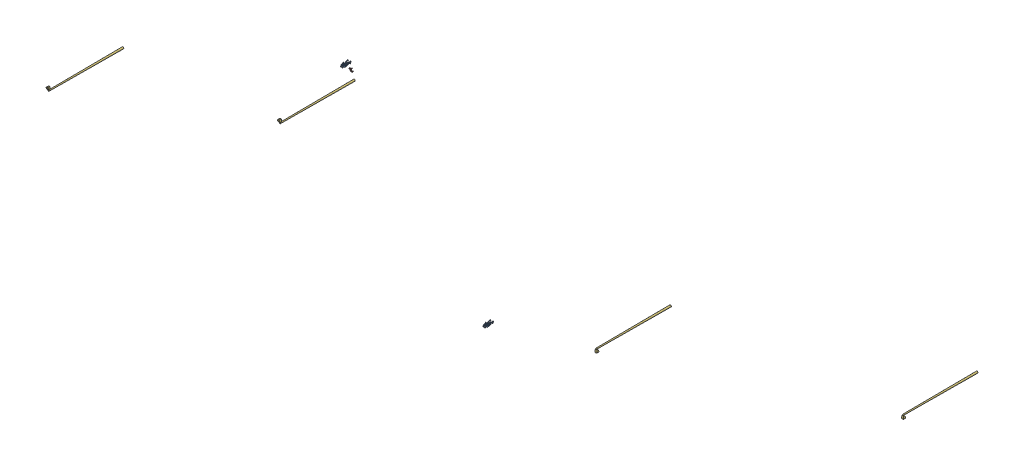
SolidWorks assembly Park scene, configuration Default. Lengths in mm.
Overall size (172997.33 40708.96 15155.93).
7 component instances, 3 part files, 8 mates.
Components (placement in the parent):
- Couple Walking v2-1: Couple Walking v2 [Default] at (97042.8871 20768.0893 0) size (971.22 682.9 1718.91)
- Couple Walking v2-2: Couple Walking v2 [Default] at (68307.1667 51803.1052 0) size (971.22 682.9 1718.91)
- German Shepherd-1: German Shepherd [Predeterminado] at (69037.0009 50613.5051 -995.4825) x (-0.927424 -0.373877 -0.010044) z (-0.373704 0.927415 -0.015684) size (212.95 642.55 996.13)
- LightPole-1: LightPole [Default] at (22635.286 31390.4456 0) x (-0.361809 0.932252 0) z (0 0 1) size (771.46 400 15150.67)
- LightPole-2: LightPole [Default] at (69285.9057 49048.0785 0) x (-0.361809 0.932252 0) z (0 0 1) size (771.46 400 15150.67)
- LightPole-3: LightPole [Default] at (133048.7527 41507.2409 0) x (0.217287 -0.976108 0) z (0 0 1) size (771.46 400 15150.67)
- LightPole-4: LightPole [Default] at (194905.5352 60880.401 0) x (0.217287 -0.976108 0) z (0 0 1) size (771.46 400 15150.67)
Mates (geometry in assembly coordinates):
- Coincident1: coincident anti-aligned: plane of Viaduct-1 through (121720.7023 -158145.4536 0) normal (0 0 -1)
- Coincident3: coincident: point of Viaduct-1
- Parallel1: parallel anti-aligned: plane of Viaduct-1 through (127159.1693 53321.2792 3923.6765) normal (0 -1 0)
- Coincident5: coincident aligned: plane of Couple Walking v2-1 through (97042.8871 20768.0893 0) normal (0 0 1)
- Coincident6: coincident aligned: plane of Couple Walking v2-2 through (68307.1667 51803.1052 0) normal (0 0 1)
- Tangent3: tangent anti-aligned: plane of Couple Walking v2-2 through (68307.1667 51803.1052 0) normal (0 0 1); face of German Shepherd-1
- Coincident7: coincident aligned: plane of LightPole-1 through (22635.286 31390.4456 0) normal (0 0 1)
- Coincident14: coincident aligned: plane of LightPole-3 through (133048.7527 41507.2409 0) normal (0 0 1)
